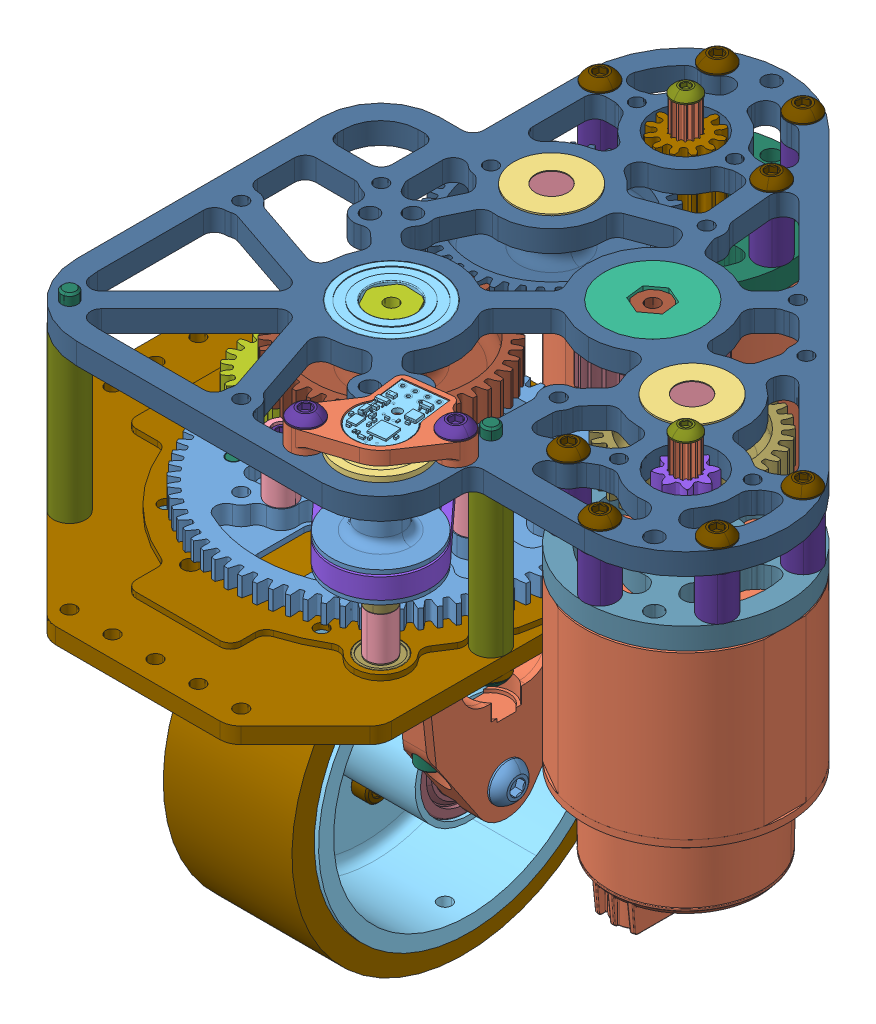
SolidWorks assembly WCP-0361 - Swerve X (Tube Mount, Flipped Gears Below).step, configuration Default. Lengths in mm.
Overall size (208.72 187.04 207.33).
106 component instances, 62 part files, 0 mates.
Components (placement in the parent):
- WCP-0364 Rev1 - WCP X Wheel Module.step-1: WCP-0364 Rev1 - WCP X Wheel Module.step [Default] at (0 -0.825 0) size (95.62 174.69 138.06)
  - WCP-0364-001 Rev1.step-1: WCP-0364-001 Rev1.step [Default] at (0 6.35 0) size (93.93 9.53 93.93)
  - WCP-0366 Rev1_Default_As Machined_.step-1: WCP-0366 Rev1_Default_As Machined_.step [Default] at (-29.2862 -49.2125 0) x (0 0 1) z (-1 0 0) size (51.81 60.46 9.5)
  - WCP-0366 Rev1_Default_As Machined_.step-2: WCP-0366 Rev1_Default_As Machined_.step [Default] at (29.2862 -49.2125 0) x (0 0 -1) z (1 0 0) size (51.81 60.46 9.5)
  - WCP-0364-006 Rev1.step-1: WCP-0364-006 Rev1.step [Default] at (0 -49.2125 0) x (1 0 0) z (0 -0.837962 0.545729) size (56.46 12.67 12.67)
  - WCP-0364-005 Rev2.step-1: WCP-0364-005 Rev2.step [Default] at (-29.2862 -1.2827 0) x (0 -1 0) z (0 0 1) size (54.08 11 11)
  - WCP-0365 Rev2.step-1: WCP-0365 Rev2.step [Default] at (2.3061 -49.2125 0) x (0 -0.866025 -0.5) z (1 0 0) size (88.9 88.9 41.15)
  - WCP-0233 Rev1.step-1: WCP-0233 Rev1.step [Default] at (-18.0375 -49.2125 0) x (0 0 -1) z (0 1 0) size (68.52 16.32 68.56)
  - WCP-0364-002 Rev1.step-1: WCP-0364-002 Rev1.step [Default] at (0 34.5757 0) x (0 -1 0) z (0.999257 0 0.03854) size (51.69 15 15)
  - WCP-0276 Rev1.step-1: WCP-0276 Rev1.step [Default] at (-29.2862 -15.4625 0) x (0 0 1) z (1 0 0) size (25.2 12.86 25.34)
  - WCP-0364-008 Rev1.step-1: WCP-0364-008 Rev1.step [Default] at (2.3061 -49.2125 0) x (1 0 0) z (0 -0.875379 0.483438) size (38.1 101.6 101.6)
  - WCP-0357 Rev1.step-1: WCP-0357 Rev1.step [Default] at origin size (88.91 6.35 88.9)
  - 217-5829_0375_flanged_thunderhex_bearing.step-1: 217-5829_0375_flanged_thunderhex_bearing.step [Default] at (-29.2862 12.7 0) x (0 -1 0) z (0.985997 0 0.166765) size (7.11 24.61 24.61)
  - 217-3489_0_250_radial_bearing.step-1: 217-3489_0_250_radial_bearing.step [Default] at (-29.2862 -29.3687 0) x (0 -1 0) z (0.460874 0 0.887465) size (4.76 12.7 12.7)
  - 217-3109_0_500_radial_bearing.step-1: 217-3109_0_500_radial_bearing.step [Default] at (18.0604 -49.2125 0) x (1 0 0) z (0 -0.205758 0.978603) size (7.94 28.57 28.57)
  - 217-3109_0_500_radial_bearing.step-2: 217-3109_0_500_radial_bearing.step [Default] at (-17.8424 -49.2125 0) x (1 0 0) z (0 0.040496 0.99918) size (7.94 28.57 28.57)
  - 217-2731_0_500_flanged_bearing.step-1: 217-2731_0_500_flanged_bearing.step [Default] at (0 4.7625 0) x (0.999376 0 -0.035335) z (0.035335 0 0.999376) size (31.12 7.94 31.12)
  - NFS-0018_SHCS_#10-32_1_750L_Default_As Machined_.step-1: NFS-0018_SHCS_#10-32_1_750L_Default_As Machined_.step [Default] at (29.2862 11.1125 17.4625) x (0.988526 0 -0.151053) z (0 1 0) size (7.92 7.92 49.28)
  - NFS-0018_SHCS_#10-32_1_750L_Default_As Machined_.step-2: NFS-0018_SHCS_#10-32_1_750L_Default_As Machined_.step [Default] at (29.2862 11.1125 -17.4625) x (0.988526 0 -0.151053) z (0 1 0) size (7.92 7.92 49.28)
  - NFS-0018_SHCS_#10-32_1_750L_Default_As Machined_.step-3: NFS-0018_SHCS_#10-32_1_750L_Default_As Machined_.step [Default] at (-29.2862 11.1125 17.4625) x (0.988526 0 -0.151053) z (0 1 0) size (7.92 7.92 49.28)
  - NFS-0018_SHCS_#10-32_1_750L_Default_As Machined_.step-4: NFS-0018_SHCS_#10-32_1_750L_Default_As Machined_.step [Default] at (-29.2862 11.1125 -17.4625) x (0.988526 0 -0.151053) z (0 1 0) size (7.92 7.92 49.28)
  - 8-32 BHCS_0.500.step-1: 8-32 BHCS_0.500.step [Default] at (-29.2862 23.8633 0) x (0.940105 0 -0.340884) z (0.340884 0 0.940105) size (7.92 14.92 7.92)
  - NFS-0059_SHCS_#4-40_0_875L_91251A113.step-1: NFS-0059_SHCS_#4-40_0_875L_91251A113.step [Default] at (23.876 3.0654 0) x (0.520663 0 0.853762) z (0 -1 0) size (4.65 4.65 25.08)
  - NFS-0059_SHCS_#4-40_0_875L_91251A113.step-2: NFS-0059_SHCS_#4-40_0_875L_91251A113.step [Default] at (-11.938 3.0654 -20.6772) x (0.520663 0 0.853762) z (0 -1 0) size (4.65 4.65 25.08)
  - NFS-0059_SHCS_#4-40_0_875L_91251A113.step-3: NFS-0059_SHCS_#4-40_0_875L_91251A113.step [Default] at (-11.938 3.0654 20.6772) x (0.520663 0 0.853762) z (0 -1 0) size (4.65 4.65 25.08)
  - 10-32 SHCS - No Thread_0.375.step-1: 10-32 SHCS - No Thread_0.375.step [Default] at (-8.2862 -69.85 0) x (0 0.591573 -0.806252) z (0 -0.806252 -0.591573) size (7.67 14.35 7.67)
  - 10-32 SHCS - No Thread_0.375.step-2: 10-32 SHCS - No Thread_0.375.step [Default] at (-8.2862 -38.8937 17.8726) x (0 -0.796051 -0.60523) z (0 -0.60523 0.796051) size (7.67 14.35 7.67)
  - 10-32 SHCS - No Thread_0.375.step-3: 10-32 SHCS - No Thread_0.375.step [Default] at (-8.2862 -59.5312 17.8726) x (0 -0.796051 -0.60523) z (0 -0.60523 0.796051) size (7.67 14.35 7.67)
  - 10-32 SHCS - No Thread_0.375.step-4: 10-32 SHCS - No Thread_0.375.step [Default] at (-8.2862 -59.5312 -17.8726) x (0 -0.796051 -0.60523) z (0 -0.60523 0.796051) size (7.67 14.35 7.67)
  - 10-32 SHCS - No Thread_0.375.step-5: 10-32 SHCS - No Thread_0.375.step [Default] at (-8.2862 -38.8937 -17.8726) x (0 -0.796051 -0.60523) z (0 -0.60523 0.796051) size (7.67 14.35 7.67)
  - 10-32 SHCS - No Thread_0.375.step-6: 10-32 SHCS - No Thread_0.375.step [Default] at (-8.2862 -28.575 0) x (0 -0.796051 -0.60523) z (0 -0.60523 0.796051) size (7.67 14.35 7.67)
  - 0250-20_3L_BHCS_91255A549.step-1: 0250-20_3L_BHCS_91255A549.step [Default] at (37.389 -49.2125 0) x (0 -0.28661 -0.958047) z (1 0 0) size (11.1 11.1 79.56)
  - NFS-0024_250-20_thin_locknut_90566A029.step-1: NFS-0024_250-20_thin_locknut_90566A029.step [Default] at (-34.0362 -49.2125 0) x (0 0.824738 0.565516) z (0 -0.565516 0.824738) size (11.14 5.19 12.86)
  - WCP-0229 Rev1.step-1: WCP-0229 Rev1.step [Default] at (-22.6822 -49.2125 0) size (0.89 16.1 14.34)
  - WCP-0229 Rev1.step-2: WCP-0229 Rev1.step [Default] at (22.6822 -49.2125 0) size (0.89 16.1 14.34)
  - WCP-0367-002 Rev3.step-1: WCP-0367-002 Rev3.step [Default] at (0 28.6559 0) x (0 0 -1) z (1 0 0) size (49.74 26.04 44.2)
  - WCP-0367-006 Rev1.step-1: WCP-0367-006 Rev1.step [Default] at (-29.2862 -3.81 0) size (17.27 17.14 17.27)
  - WCP-0367-010 Rev1.step-1: WCP-0367-010 Rev1.step [Default] at (-29.2862 22.2758 0) x (0 0 1) z (-1 0 0) size (12.7 3.97 12.7)
  - WCP-0434 Rev1.step-1: WCP-0434 Rev1.step [Default] at (-29.2862 19 0) x (-0.327758 0 -0.944762) z (0 -1 0) size (30.3 30.48 12.6)
  - 217-5464_24T_500_hex_steel.step-1: 217-5464_24T_500_hex_steel.step [Default] at (0 19 0) x (0.428371 0 0.903603) z (0 -1 0) size (32.87 32.87 12.6)
- WCP-0360-001 Rev1.step-1: WCP-0360-001 Rev1.step [Default] at origin size (133.35 8 133.35)
- WCP-0361-001 Rev2.step-1: WCP-0361-001 Rev2.step [Default] at (0 53.1812 0) size (174.12 6.35 174.12)
- WCP-0364-003 Rev1.step-1: WCP-0364-003 Rev1.step [Default] at (38.669 7.5147 -38.669) x (0.682654 0 0.730742) z (0 1 0) size (20.01 20.32 56.54)
- WCP-0364-004 Rev1.step-1: WCP-0364-004 Rev1.step [Default] at (36.5633 23.984 39.7383) x (0 1 0) z (-0.373833 0 -0.927496) size (58.72 11 11)
- WCP-0361-004 Rev1_Default_As Machined_.step-1: WCP-0361-004 Rev1_Default_As Machined_.step [Default] at (69.0125 43.1356 -19.9819) x (0 -1 0) z (-0.01804 0 -0.999837) size (25.16 11 11)
- WCP-0361-004 Rev1_Default_As Machined_.step-2: WCP-0361-004 Rev1_Default_As Machined_.step [Default] at (-5.7166 43.1356 -53.1094) x (0 -1 0) z (0.932067 0 0.362285) size (25.16 11 11)
- WCP-0361-005 Rev1.step-1: WCP-0361-005 Rev1.step [Default] at (86.9695 34.1313 -0.16) x (0.741112 0 -0.671382) z (0.671382 0 0.741112) size (60 6.35 71.67)
- WCP-0361-002 Rev1.step-1: WCP-0361-002 Rev1.step [Default] at (0.16 34.1313 -86.9695) x (-0.985271 0 -0.170999) z (0.170999 0 -0.985271) size (60 6.35 79.29)
- WCP-0387 Rev1.step-1: WCP-0387 Rev1.step [Default] at (-47.625 26.1937 47.625) x (0 -1 0) z (-0.427741 0 0.903901) size (47.62 9.5 9.5)
- WCP-0387 Rev1.step-2: WCP-0387 Rev1.step [Default] at (49.2125 26.1937 19.7361) x (0 -1 0) z (0.97467 0 0.223647) size (47.62 9.5 9.5)
- WCP-0202 Rev1.step-1: WCP-0202 Rev1.step [Default] at (64.9724 43.6562 12.54) x (0 -1 0) z (0.721842 0 0.692058) size (12.7 9.5 9.5)
- WCP-0202 Rev1.step-2: WCP-0202 Rev1.step [Default] at (108.9665 43.6562 -12.86) x (0 -1 0) z (0.721842 0 0.692058) size (12.7 9.5 9.5)
- WCP-0202 Rev1.step-3: WCP-0202 Rev1.step [Default] at (86.9695 43.6562 25.24) x (0 -1 0) z (0.721842 0 0.692058) size (12.7 9.5 9.5)
- WCP-0202 Rev1.step-4: WCP-0202 Rev1.step [Default] at (108.9665 43.6562 12.54) x (0 -1 0) z (0.721842 0 0.692058) size (12.7 9.5 9.5)
- WCP-0202 Rev1.step-5: WCP-0202 Rev1.step [Default] at (25.56 43.6562 -86.9695) x (0 -1 0) z (0.721842 0 0.692058) size (12.7 9.5 9.5)
- WCP-0202 Rev1.step-6: WCP-0202 Rev1.step [Default] at (12.86 43.6562 -108.9665) x (0 -1 0) z (0.721842 0 0.692058) size (12.7 9.5 9.5)
- WCP-0202 Rev1.step-7: WCP-0202 Rev1.step [Default] at (-12.54 43.6562 -108.9665) x (0 -1 0) z (0.721842 0 0.692058) size (12.7 9.5 9.5)
- WCP-0202 Rev1.step-8: WCP-0202 Rev1.step [Default] at (-25.24 43.6562 -86.9695) x (0 -1 0) z (0.721842 0 0.692058) size (12.7 9.5 9.5)
- WCP-0226 Rev1.step-1: WCP-0226 Rev1.step [Default] at (-19.7361 16.6687 -49.2125) x (0 1 0) z (0.900957 0 0.433909) size (28.57 9.5 9.5)
- WCP-0307 Rev1.step-1: WCP-0307 Rev1.step [Default] at (-19.7361 -5.5913 -49.2125) x (0 -1 0) z (-0.403935 0 0.914788) size (3.18 9.5 9.5)
- 217-6515_Falcon_500_Default_As Machined_.step-1: 217-6515_Falcon_500_Default_As Machined_.step [Default] at (0.16 4.7562 -86.9695) x (0.5 0 0.866025) z (0 1 0) size (60 60 115.81)
- 217-6515_Falcon_500_Default_As Machined_.step-2: 217-6515_Falcon_500_Default_As Machined_.step [Default] at (86.9695 4.7562 -0.16) x (0.866025 0 -0.5) z (0 1 0) size (60 60 115.81)
- 217-2733_0_375_flanged_bearing.step-1: 217-2733_0_375_flanged_bearing.step [Default] at (36.5633 57.9438 39.7383) x (0 -1 0) z (0.710471 0 -0.703726) size (7.11 24.61 24.61)
- 217-3489_0_250_radial_bearing.step-1: 217-3489_0_250_radial_bearing.step [Default] at (36.5633 1.6187 39.7383) x (0 1 0) z (-0.269707 0 0.962942) size (4.76 12.7 12.7)
- WCP-0041_0_250_radial_bearing.step-1: WCP-0041_0_250_radial_bearing.step [Default] at (38.669 1.5108 -38.669) x (-0.316483 0 0.948598) z (0 -1 0) size (15.88 15.88 4.98)
- 217-4006_0_500_flanged_thunderhex_bearing.step-1: 217-4006_0_500_flanged_thunderhex_bearing.step [Default] at (0 52.3875 0) x (-0.903668 0 0.428233) z (0 -1 0) size (31.12 31.12 7.94)
- 217-2735_0_375_flanged_hex_bearing.step-1: 217-2735_0_375_flanged_hex_bearing.step [Default] at (38.669 56.3562 -38.669) x (-0.91814 0 -0.396256) z (-0.396256 0 0.91814) size (31.12 7.94 31.12)
- 217-2733_0_375_flanged_bearing.step-2: 217-2733_0_375_flanged_bearing.step [Default] at (69.0125 49.6887 -19.9819) x (0 1 0) z (0.053261 0 -0.998581) size (7.11 24.61 24.61)
- 217-2733_0_375_flanged_bearing.step-3: 217-2733_0_375_flanged_bearing.step [Default] at (-5.7166 49.6887 -53.1094) x (0 1 0) z (0.053261 0 -0.998581) size (7.11 24.61 24.61)
- WCP-0042_0_250_flanged_bearing.step-1: WCP-0042_0_250_flanged_bearing.step [Default] at (69.0125 33.8899 -19.9819) x (0.753109 0 -0.657896) z (0 1 0) size (18.24 18.24 4.98)
- WCP-0042_0_250_flanged_bearing.step-2: WCP-0042_0_250_flanged_bearing.step [Default] at (-5.7166 33.8899 -53.1094) x (0.890667 0 -0.454657) z (0 1 0) size (18.24 18.24 4.98)
- 217-6915_Falcon_8T.step-1: 217-6915_Falcon_8T.step [Default] at (86.9695 46.7088 -0.16) x (0.340812 0 -0.940132) z (0 -1 0) size (13.62 13.62 19.06)
- 217-6919_Falcon_12T.step-1: 217-6919_Falcon_12T.step [Default] at (0.16 46.7088 -86.9695) x (-0.557793 0 0.82998) z (0 -1 0) size (17.78 17.78 19.05)
- WCP-0541 Rev1.step-1: WCP-0541 Rev1.step [Default] at (-5.7166 43.1482 -53.1094) x (0.992001 0 0.126228) z (0 1 0) size (55.8 55.88 12.65)
- WCP-0178 Rev1.step-1: WCP-0178 Rev1.step [Default] at (0 42.0941 0) x (0.993242 0 -0.116064) z (0 1 0) size (55.8 55.88 12.65)
- WCP-0540 Rev1.step-1: WCP-0540 Rev1.step [Default] at (69.0125 43.1236 -19.9819) x (0.992415 0 -0.122933) z (0 1 0) size (43.07 43.07 12.6)
- WCP-0538 Rev1.step-1: WCP-0538 Rev1.step [Default] at (38.669 41.9158 -38.669) x (0.27049 0 -0.962723) z (0 1 0) size (32.86 32.86 12.65)
- 10-32 BHCS - No Thread_0.250.step-1: 10-32 BHCS - No Thread_0.250.step [Default] at (-33.4155 -4 33.4155) x (0.140263 0 -0.990114) z (-0.990114 0 -0.140263) size (9.17 8.92 9.17)
- 10-32 BHCS - No Thread_2.500.step-1: 10-32 BHCS - No Thread_2.500.step [Default] at (-47.625 -4 47.625) x (0.958479 0 -0.285162) z (-0.285162 0 -0.958479) size (9.17 66.07 9.17)
- 10-32 BHCS - No Thread_2.500.step-2: 10-32 BHCS - No Thread_2.500.step [Default] at (49.2125 -4 19.7361) x (0.670106 0 -0.742266) z (-0.742266 0 -0.670106) size (9.17 66.07 9.17)
- 10-32 BHCS - No Thread_1.750.step-1: 10-32 BHCS - No Thread_1.750.step [Default] at (-19.7361 -7.175 -49.2125) x (0.978856 0 -0.204553) z (-0.204553 0 -0.978856) size (9.17 47.02 9.17)
- 10-32 BHCS - No Thread_0.500.step-1: 10-32 BHCS - No Thread_0.500.step [Default] at (23.914 62.9348 49.3306) x (-0.153016 0 -0.988224) z (0.988224 0 -0.153016) size (9.17 15.27 9.17)
- 10-32 BHCS - No Thread_0.500.step-2: 10-32 BHCS - No Thread_0.500.step [Default] at (49.2125 62.9348 30.146) x (0.162273 0 -0.986746) z (0.986746 0 0.162273) size (9.17 15.27 9.17)
- 8-32 BHCS_0.500.step-1: 8-32 BHCS_0.500.step [Default] at (86.9695 65.7588 -0.16) x (-0.999431 0 -0.033743) z (0.033743 0 -0.999431) size (7.92 14.92 7.92)
- 8-32 BHCS_0.500.step-2: 8-32 BHCS_0.500.step [Default] at (0.16 65.7588 -86.9695) x (0.994914 0 -0.100726) z (0.100726 0 0.994914) size (7.92 14.92 7.92)
- 10-32 BHCS - No Thread_1.250.step-1: 10-32 BHCS - No Thread_1.250.step [Default] at (64.9724 56.3562 12.54) x (0.165498 0 -0.98621) z (0.98621 0 0.165498) size (9.17 34.32 9.17)
- 10-32 BHCS - No Thread_1.250.step-2: 10-32 BHCS - No Thread_1.250.step [Default] at (108.9665 56.3562 -12.86) x (-0.767084 0 0.641546) z (-0.641546 0 -0.767084) size (9.17 34.32 9.17)
- 10-32 BHCS - No Thread_1.250.step-3: 10-32 BHCS - No Thread_1.250.step [Default] at (108.9665 56.3562 12.54) x (0.162273 0 -0.986746) z (0.986746 0 0.162273) size (9.17 34.32 9.17)
- 10-32 BHCS - No Thread_1.250.step-4: 10-32 BHCS - No Thread_1.250.step [Default] at (86.9695 56.3562 25.24) x (0.162273 0 -0.986746) z (0.986746 0 0.162273) size (9.17 34.32 9.17)
- 10-32 BHCS - No Thread_1.250.step-5: 10-32 BHCS - No Thread_1.250.step [Default] at (25.56 56.3562 -86.9695) x (-0.843804 0 0.536652) z (-0.536652 0 -0.843804) size (9.17 34.32 9.17)
- 10-32 BHCS - No Thread_1.250.step-6: 10-32 BHCS - No Thread_1.250.step [Default] at (-12.54 56.3562 -108.9665) x (0.93512 0 0.354332) z (-0.354332 0 0.93512) size (9.17 34.32 9.17)
- 10-32 BHCS - No Thread_1.250.step-7: 10-32 BHCS - No Thread_1.250.step [Default] at (-25.24 56.3562 -86.9695) x (0.162273 0 -0.986746) z (0.986746 0 0.162273) size (9.17 34.32 9.17)
- 10-32 BHCS - No Thread_1.250.step-8: 10-32 BHCS - No Thread_1.250.step [Default] at (12.86 56.3562 -108.9665) x (0.162273 0 -0.986746) z (0.986746 0 0.162273) size (9.17 34.32 9.17)
- WCP-0367-003 Rev2.step-1: WCP-0367-003 Rev2.step [Default] at (36.5633 25.8309 39.7383) x (-0.999998 0 0.001857) z (0 -1 0) size (29.05 29.05 26.83)
- WCP-0367-012 Rev1_30 Left.step-1: WCP-0367-012 Rev1_30 Left.step [Default] at (36.5633 60.9155 39.7383) x (-0.992171 0 0.124885) z (-0.124885 0 -0.992171) size (37.02 6.58 29.76)
- WCP-0367-001 Rev1.step-1: WCP-0367-001 Rev1.step [Default] at (0 35.3446 0) x (0.987744 0 0.156082) z (-0.156082 0 0.987744) size (19.05 0.51 19.05)
- WCP-0367-004 Rev1.step-1: WCP-0367-004 Rev1.step [Default] at (36.5633 10.35 39.7383) size (8 12.7 8)
- 10-32 BHCS - No Thread_0.250.step-2: 10-32 BHCS - No Thread_0.250.step [Default] at (-42.106 -4 -21.4541) x (0.984998 0 -0.172564) z (-0.172564 0 -0.984998) size (9.17 8.92 9.17)
- 10-32 BHCS - No Thread_0.250.step-3: 10-32 BHCS - No Thread_0.250.step [Default] at (7.3926 -4 -46.6749) x (0.4685 0 0.883464) z (0.883464 0 -0.4685) size (9.17 8.92 9.17)
- 10-32 BHCS - No Thread_0.250.step-4: 10-32 BHCS - No Thread_0.250.step [Default] at (46.6749 -4 -7.3926) x (-0.69545 0 0.718575) z (0.718575 0 0.69545) size (9.17 8.92 9.17)
- 10-32 BHCS - No Thread_0.250.step-5: 10-32 BHCS - No Thread_0.250.step [Default] at (21.4541 -4 42.106) x (-0.898311 0 -0.43936) z (-0.43936 0 0.898311) size (9.17 8.92 9.17)
- CANcoder.step-1: CANcoder.step [Default] at (36.5485 59.1546 39.7225) x (-0.992171 0 0.124885) z (0 1 0) size (15.94 23.28 4.54)
- WCP-0156 Rev1.step-1: WCP-0156 Rev1.step [Default] at (36.5633 51.5938 39.7383) size (6.35 12.7 6.35)
- Falcon_Motor_Spacer_0625.step-1: Falcon_Motor_Spacer_0625.step [Default] at (86.9695 36.39 -0.16) size (12.7 1.59 12.7)
- Falcon_Motor_Spacer_0625.step-2: Falcon_Motor_Spacer_0625.step [Default] at (0.16 36.39 -86.9695) x (0.98238 0 0.186896) z (-0.186896 0 0.98238) size (12.7 1.59 12.7)
- Encoder Belt.step-1: Encoder Belt.step [Default] at (18.2816 30.8309 19.8691) x (0.677097 0 0.735894) z (-0.735894 0 0.677097) size (83.28 6 29.28)
